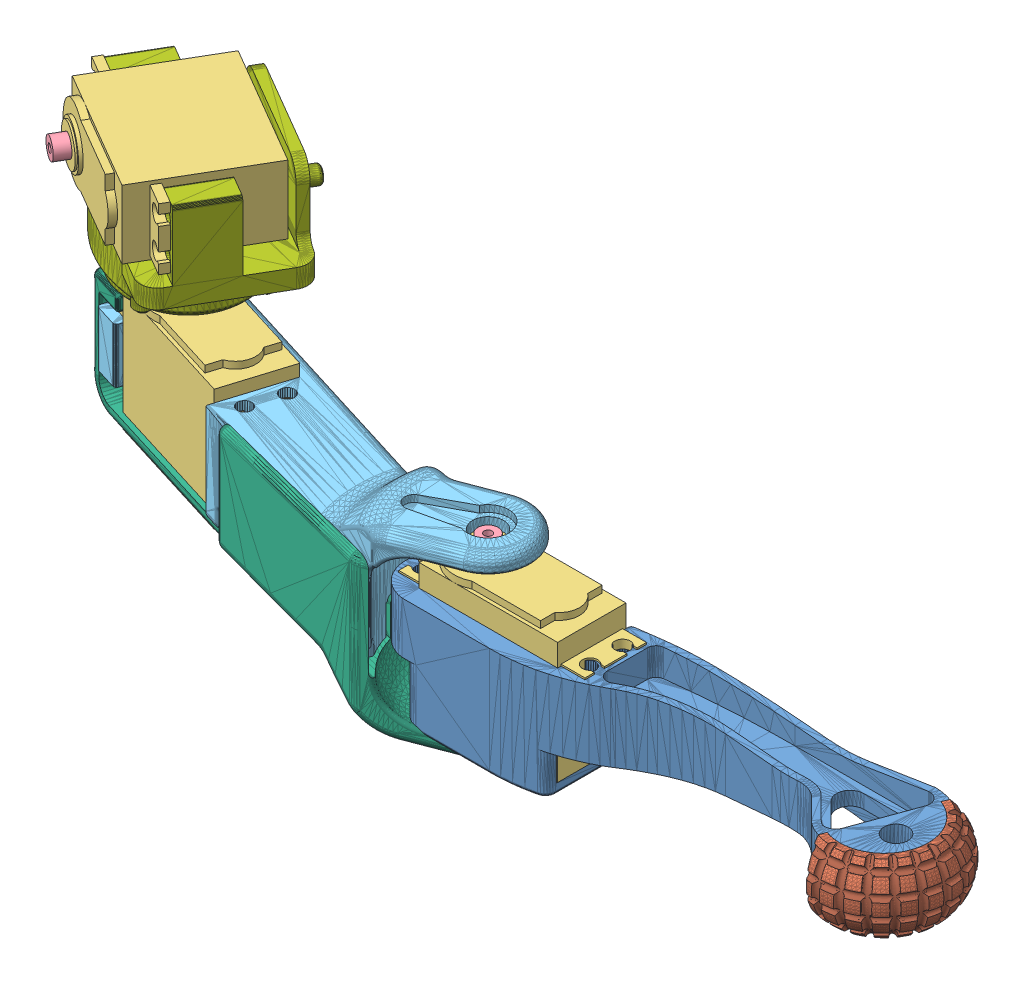
SolidWorks assembly left_foot_back, configuration Default. Lengths in mm.
Overall size (284.28 93.4 85.82).
14 component instances, 7 part files, 23 mates.
Components (placement in the parent):
- L_wrist_mg-1: L_wrist_mg [Default] at (-104.9134 49.2874 139.9903) size (149.99 36.9 30)
- foot-1: foot [Default] at (21.0866 19.2874 149.9903) x (0.342019 0 -0.939693) z (-0.939693 0 -0.342019) size (38.32 20 19.41)
- MG996R-1: MG996R [Default] at (-84.6634 -9.7126 149.9903) size (54.5 43 20)
  - servo-1: servo [Default] at origin size (54.5 39 20)
  - shaft-1: shaft [Default] at (-10.1089 43 0) x (-0.837169 0 -0.546944) z (-0.546944 0 0.837169) size (5.9 19.57 5.9)
- L_arm_mg-1: L_arm_mg [Default] at (-207.5786 26.2874 118.9596) x (-0.296504 0 0.955032) z (0.955032 0 0.296504) size (38.24 39.8 137.4)
- MG996R-2: MG996R [Default] at (-191.2042 -5.7126 134.5142) x (0.955032 0 0.296504) z (-0.296504 0 0.955032) size (54.5 43 20)
  - servo-1: servo [Default] at origin size (54.5 39 20)
  - shaft-1: shaft [Default] at (-10.1089 43 0) x (-0.837169 0 -0.546944) z (-0.546944 0 0.837169) size (5.9 19.57 5.9)
- L_arm_cover-1: L_arm_cover [Default] at (-212.633 28.5874 111.6314) x (-0.296504 0 0.955032) z (0.955032 0 0.296504) size (41.16 45 143.55)
- L_arm_joint_mg-1: L_arm_joint_mg [Default] at (-178.2705 74.7874 132.9075) x (0 -1 0) z (-0.863446 0 -0.504441) size (37.5 46 56.5)
- MG996R-3: MG996R [Default] at (-193.5921 65.7874 117.0074) x (0.863446 0 0.504441) z (0 -1 0) size (54.5 43 20)
  - servo-1: servo [Default] at origin size (54.5 39 20)
  - shaft-1: shaft [Default] at (-10.1089 43 0) x (-0.837169 0 -0.546944) z (-0.546944 0 0.837169) size (5.9 19.57 5.9)
Mates (geometry in assembly coordinates):
- Coincident1: coincident anti-aligned: plane of L_wrist_mg-1 through (9.5615 49.2874 181.6556) normal (0.939693 0 0.342019); plane of foot-1 through (21.0866 19.2874 149.9903) normal (-0.939693 0 -0.342019)
- Parallel2: parallel aligned: line of foot-1 through (16.6404 -0.7126 162.2063) axis (0 1 0); line of L_wrist_mg-1 through (16.6404 -0.7126 162.2063) axis (0 1 0)
- Coincident4: coincident: point of foot-1; point of L_wrist_mg-1
- Coincident5: coincident anti-aligned: plane of L_wrist_mg-1 through (-104.9134 49.2874 159.9903) normal (0 0 -1); plane of MG996R-1/servo-1 through (-104.9134 25.7874 159.9903) normal (0 0 1)
- Coincident6: coincident anti-aligned: plane of L_wrist_mg-1 through (-104.9134 -9.7126 139.9903) normal (0 1 0); plane of MG996R-1/servo-1 through (-84.6634 -9.7126 149.9903) normal (0 -1 0)
- Coincident7: coincident anti-aligned: plane of L_wrist_mg-1 through (-64.4134 49.2874 139.9903) normal (-1 0 0); plane of MG996R-1/servo-1 through (-64.4134 25.7874 159.9903) normal (1 0 0)
- Parallel4: parallel aligned: plane of MG996R-1/servo-1 through (-94.7723 27.7874 149.9903) normal (0 1 0); plane of L_arm_mg-1 through (-207.5786 26.2874 118.9596) normal (0 1 0)
- Coincident14: coincident anti-aligned: plane of L_arm_mg-1 through (-207.5786 21.2874 118.9596) normal (0 1 0); plane of MG996R-2/servo-1 through (-213.1941 21.2874 122.7134) normal (0 -1 0)
- Coincident15: coincident anti-aligned: plane of L_arm_mg-1 through (-207.5786 26.2874 118.9596) normal (0.955032 0 0.296504); plane of MG996R-2/servo-1 through (-213.5086 29.7874 138.0603) normal (-0.955032 0 -0.296504)
- Coincident16: coincident anti-aligned: plane of L_arm_mg-1 through (-207.5786 26.2874 118.9596) normal (-0.296504 0 0.955032); plane of MG996R-2/servo-1 through (-207.5786 29.7874 118.9596) normal (0.296504 0 -0.955032)
- Coincident18: coincident: line of MG996R-1/shaft-1 through (-94.7723 33.2874 149.9903) axis (0 -1 0)
- Distance1: distance = 2 mm: line of L_arm_mg-1 through (-92.1971 31.2874 153.6666) axis (-0.573724 0 -0.819049)
- Coincident21: coincident anti-aligned: plane of L_arm_cover-1 through (-212.633 23.7874 111.6314) normal (0 -1 0); plane of MG996R-2/servo-1 through (-213.1941 23.7874 122.7134) normal (0 1 0)
- Parallel5: parallel anti-aligned: plane of MG996R-2/servo-1 through (-213.5086 29.7874 138.0603) normal (-0.955032 0 -0.296504); plane of L_arm_cover-1 through (-205.9478 28.5874 113.707) normal (0.955032 0 0.296504)
- Coincident23: coincident anti-aligned: plane of MG996R-2/servo-1 through (-213.5086 29.7874 138.0603) normal (-0.955032 0 -0.296504); plane of L_arm_cover-1 through (-205.9478 28.5874 113.707) normal (0.955032 0 0.296504)
- Parallel6: parallel aligned: plane of L_arm_mg-1 through (-206.096 26.2874 114.1845) normal (0.296504 0 -0.955032); plane of L_arm_cover-1 through (-212.633 28.5874 111.6314) normal (0.296504 0 -0.955032)
- Coincident25: coincident anti-aligned: plane of L_arm_mg-1 through (-207.5786 26.2874 118.9596) normal (-0.296504 0 0.955032); plane of L_arm_cover-1 through (-214.2638 28.5874 116.8841) normal (0.296504 0 -0.955032)
- Parallel7: parallel aligned: plane of MG996R-2/shaft-1 through (-200.8585 37.2874 131.5168) normal (0 1 0); plane of L_arm_joint_mg-1 through (-178.2705 54.7874 132.9075) normal (0 1 0)
- Coincident27: coincident: line of MG996R-2/shaft-1 through (-200.8585 37.2874 131.5168) axis (0 -1 0)
- Coincident28: coincident anti-aligned: plane of MG996R-2/shaft-1 through (-200.8585 37.2874 131.5168) normal (0 1 0); plane of L_arm_joint_mg-1 through (-178.2705 37.2874 132.9075) normal (0 -1 0)
- Coincident29: coincident anti-aligned: plane of L_arm_joint_mg-1 through (-188.8638 74.7874 151.0398) normal (-0.504441 0 0.863446); plane of MG996R-3/servo-1 through (-228.3665 70.5374 127.9617) normal (0.504441 0 -0.863446)
- Coincident30: coincident aligned: plane of L_arm_joint_mg-1 through (-220.1477 74.7874 108.4421) normal (-0.863446 0 -0.504441); plane of MG996R-3/servo-1 through (-230.7409 72.0374 126.5745) normal (-0.863446 0 -0.504441)
- Coincident31: coincident aligned: plane of L_arm_joint_mg-1 through (-178.2705 74.7874 132.9075) normal (0 1 0); plane of MG996R-3/servo-1 through (-224.6968 74.7874 130.1055) normal (0 1 0)
